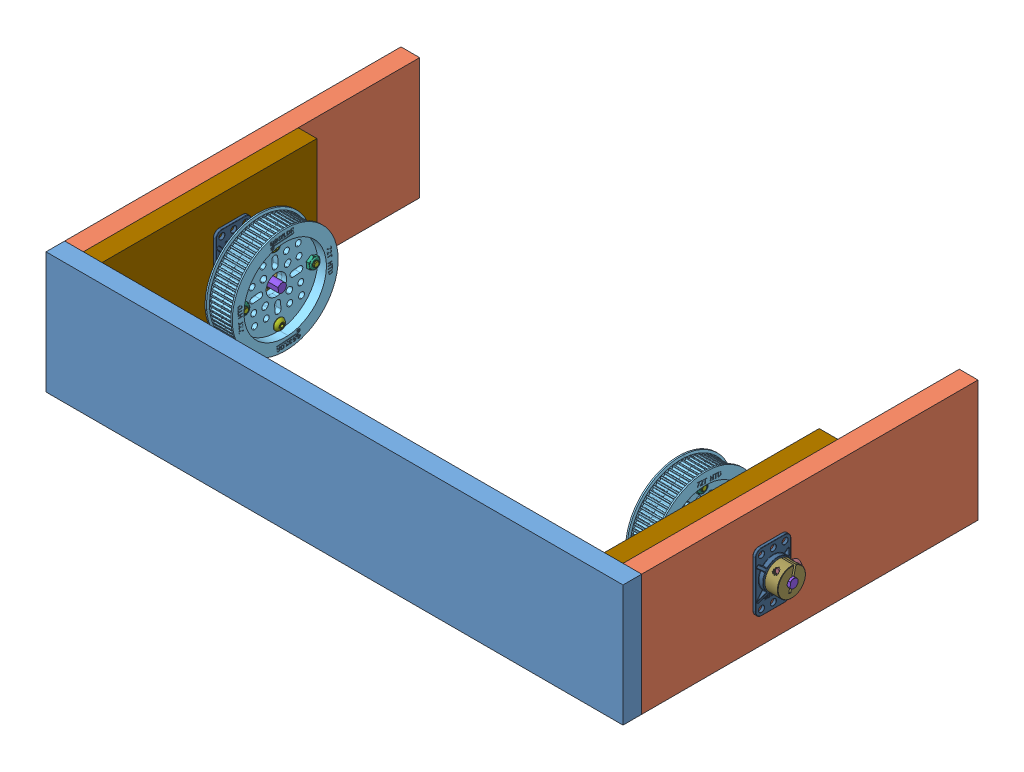
SolidWorks assembly hautElevateur, configuration Défaut. Lengths in mm.
Overall size (424.23 82.55 241.3).
75 component instances, 13 part files, 6 mates.
Components (placement in the parent):
- plaqueMoteurElevateur-1: plaqueMoteurElevateur [Défaut] at (-14.6749 -16.481 385.8661) size (392.22 82.55 12.7)
- pivotHautElevateur-1: pivotHautElevateur [Défaut] at (-183.2969 -207.8009 -55.2233) x (0 0 1) z (0 1 0) size (228.6 78.41 82.55)
  - plaqueHaut-1: plaqueHaut [Défaut] at (326.7894 -14.786 191.3199) x (1 0 0) z (0 -1 0) size (228.6 82.55 12.7)
  - 1309-0016-1006 assembly-1: 1309-0016-1006 assembly [Défaut] at (365.0893 27.1876 177.1992) x (0.655754 0 -0.754974) z (0 -1 0) size (28.36 32 10.95)
    - 1309-0016-1006 assembly.STEP-1: 1309-0016-1006 assembly.STEP [Défaut] at origin size (28.36 32 10.95)
      - 1309-0016-1006.STEP-1: 1309-0016-1006.STEP [Défaut] at (-18.2019 0.5776 8.7736) size (25.38 32 10)
      - 2800-0004-0014_90128A207.STEP-1: 2800-0004-0014_90128A207.STEP [Défaut] at (-16.149 11.6963 8.7736) x (0.5 -0.5 -0.707107) z (0.707107 0.707107 0) size (7 7 18.01)
      - 2800-0004-0014_90128A207.STEP-2: 2800-0004-0014_90128A207.STEP [Défaut] at (-20.2547 -10.5411 8.7736) x (-0.5 0.5 -0.707107) z (-0.707107 -0.707107 0) size (7 7 18.01)
  - 3402-0014-0072 pulley-1: 3402-0014-0072 pulley [Défaut] at (364.8802 56.6295 250.8953) x (0.070159 0 0.997536) z (0 -1 0) size (71.96 71.96 18.5)
    - 3402-0014-0072 assembly.STEP-1: 3402-0014-0072 assembly.STEP [Défaut] at origin size (71.96 71.96 18.5)
      - 3402-0014-0072.STEP-1: 3402-0014-0072.STEP [Défaut] at (-60.2208 7.0832 38.7155) size (71.96 71.96 10.5)
      - 3402-0014-0072.STEP-2: 3402-0014-0072.STEP [Défaut] at (-60.2208 7.0832 23.2155) x (0 -1 0) z (0 0 -1) size (71.96 71.96 10.5)
      - 2812-0004-0007_90576A103.STEP-1: 2812-0004-0007_90576A103.STEP [Défaut] at (-60.2208 31.0832 29.7155) x (0.866025 0.5 0) z (-0.5 0.866025 0) size (7.02 4.86 8.1)
      - 2812-0004-0007_90576A103.STEP-2: 2812-0004-0007_90576A103.STEP [Défaut] at (-60.2208 -16.9168 29.7155) x (0 1 0) z (-1 0 0) size (7.02 4.86 8.1)
      - 2812-0004-0007_90576A103.STEP-3: 2812-0004-0007_90576A103.STEP [Défaut] at (-84.2208 7.0832 32.2155) x (0.5 0.866025 0) z (0.866025 -0.5 0) size (7.02 4.86 8.1)
      - 2812-0004-0007_90576A103.STEP-4: 2812-0004-0007_90576A103.STEP [Défaut] at (-36.2208 7.0832 32.2155) x (1 0 0) z (0 -1 0) size (7.02 4.86 8.1)
      - 2802-0004-0010_92095A480.STEP-1: 2802-0004-0010_92095A480.STEP [Défaut] at (-36.2208 7.0832 25.5155) x (-0.923728 -0.383049 0) z (0 0 -1) size (13.53 12.99 15.57)
      - 2802-0004-0010_92095A480.STEP-2: 2802-0004-0010_92095A480.STEP [Défaut] at (-84.2208 7.0832 25.5155) x (0.923728 0.383049 0) z (0 0 -1) size (13.53 12.99 15.57)
      - 2802-0004-0010_92095A480.STEP-3: 2802-0004-0010_92095A480.STEP [Défaut] at (-60.2208 31.0832 36.4155) size (13.53 12.99 15.57)
      - 2802-0004-0010_92095A480.STEP-4: 2802-0004-0010_92095A480.STEP [Défaut] at (-60.2208 -16.9168 36.4155) x (-1 0 0) z (0 0 1) size (13.53 12.99 15.57)
  - 2101-0006-0300 3 po-1: 2101-0006-0300 3 po [Défaut] at (353.5894 -43.494 191.3199) x (0.070159 0 0.997536) z (-0.997536 0 0.070159) size (6 76.2 5.5)
  - blocHautCote-1: blocHautCote [Défaut] at (368.0644 -2.086 191.3199) x (1 0 0) z (0 -1 0) size (146.05 82.55 12.7)
  - 1616-0016-0002 plaque-1: 1616-0016-0002 plaque [Défaut] at (353.5894 -27.486 193.3199) size (24 5.02 40)
    - 1616-0016-0002.STEP-1: 1616-0016-0002.STEP [Défaut] at origin size (24 5.02 40)
      - 1616-0016-0002.STEP-1: 1616-0016-0002.STEP [Défaut] at origin size (24 5.02 40)
  - 1616-0016-0002 plaque-2: 1616-0016-0002 plaque [Défaut] at (353.5894 -2.086 193.3199) x (-1 0 0) z (0 0 1) size (24 5.02 40)
    - 1616-0016-0002.STEP-1: 1616-0016-0002.STEP [Défaut] at origin size (24 5.02 40)
      - 1616-0016-0002.STEP-1: 1616-0016-0002.STEP [Défaut] at origin size (24 5.02 40)
  - 1611-0514-0006 Roulement-1: 1611-0514-0006 Roulement [Défaut] at (353.5894 -32.486 191.3199) x (0.999897 0 0.014368) z (-0.014368 0 0.999897) size (15 5 15)
  - 2910-0919-0006 assembly collet-6: 2910-0919-0006 assembly collet [Défaut] at (379.8638 -36.9656 167.7839) x (0.972179 0 -0.234238) z (0.234238 0 0.972179) size (19 9.89 19.83)
    - 2910-0919-0006 assembly.STEP-1: 2910-0919-0006 assembly.STEP [Défaut] at origin size (19 9.89 19.83)
      - 2910-0919-0006.STEP-1: 2910-0919-0006.STEP [Défaut] at (-31.0565 -0.5204 16.7268) size (19 9.5 18.97)
      - 2800-0004-0010_90128A207.STEP-1: 2800-0004-0010_90128A207.STEP [Défaut] at (-24.2865 -0.5204 11.2868) x (0 -0.807243 -0.59022) z (1 0 0) size (7 7 14.01)
  - 1611-0514-0006 Roulement-2: 1611-0514-0006 Roulement [Défaut] at (353.5894 2.914 191.3199) x (-0.983829 0 -0.179109) z (-0.179109 0 0.983829) size (15 5 15)
  - 2910-0919-0006 assembly collet-7: 2910-0919-0006 assembly collet [Défaut] at (322.5329 7.3936 174.5931) x (-1 0 0) z (0 0 1) size (19 9.89 19.83)
    - 2910-0919-0006 assembly.STEP-1: 2910-0919-0006 assembly.STEP [Défaut] at origin size (19 9.89 19.83)
      - 2910-0919-0006.STEP-1: 2910-0919-0006.STEP [Défaut] at (-31.0565 -0.5204 16.7268) size (19 9.5 18.97)
      - 2800-0004-0010_90128A207.STEP-1: 2800-0004-0010_90128A207.STEP [Défaut] at (-24.2865 -0.5204 11.2868) x (0 -0.807243 -0.59022) z (1 0 0) size (7 7 14.01)
- pivotHautElevateur-2: pivotHautElevateur [Défaut] at (153.9472 174.8389 -55.2233) x (0 0 1) z (0 -1 0) size (228.6 78.41 82.55)
  - plaqueHaut-1: plaqueHaut [Défaut] at (326.7894 -14.786 191.3199) x (1 0 0) z (0 -1 0) size (228.6 82.55 12.7)
  - 1309-0016-1006 assembly-1: 1309-0016-1006 assembly [Défaut] at (365.0893 27.1876 177.1992) x (0.655754 0 -0.754974) z (0 -1 0) size (28.36 32 10.95)
    - 1309-0016-1006 assembly.STEP-1: 1309-0016-1006 assembly.STEP [Défaut] at origin size (28.36 32 10.95)
      - 1309-0016-1006.STEP-1: 1309-0016-1006.STEP [Défaut] at (-18.2019 0.5776 8.7736) size (25.38 32 10)
      - 2800-0004-0014_90128A207.STEP-1: 2800-0004-0014_90128A207.STEP [Défaut] at (-16.149 11.6963 8.7736) x (0.5 -0.5 -0.707107) z (0.707107 0.707107 0) size (7 7 18.01)
      - 2800-0004-0014_90128A207.STEP-2: 2800-0004-0014_90128A207.STEP [Défaut] at (-20.2547 -10.5411 8.7736) x (-0.5 0.5 -0.707107) z (-0.707107 -0.707107 0) size (7 7 18.01)
  - 3402-0014-0072 pulley-1: 3402-0014-0072 pulley [Défaut] at (364.8802 56.6295 250.8953) x (0.070159 0 0.997536) z (0 -1 0) size (71.96 71.96 18.5)
    - 3402-0014-0072 assembly.STEP-1: 3402-0014-0072 assembly.STEP [Défaut] at origin size (71.96 71.96 18.5)
      - 3402-0014-0072.STEP-1: 3402-0014-0072.STEP [Défaut] at (-60.2208 7.0832 38.7155) size (71.96 71.96 10.5)
      - 3402-0014-0072.STEP-2: 3402-0014-0072.STEP [Défaut] at (-60.2208 7.0832 23.2155) x (0 -1 0) z (0 0 -1) size (71.96 71.96 10.5)
      - 2812-0004-0007_90576A103.STEP-1: 2812-0004-0007_90576A103.STEP [Défaut] at (-60.2208 31.0832 29.7155) x (0.866025 0.5 0) z (-0.5 0.866025 0) size (7.02 4.86 8.1)
      - 2812-0004-0007_90576A103.STEP-2: 2812-0004-0007_90576A103.STEP [Défaut] at (-60.2208 -16.9168 29.7155) x (0 1 0) z (-1 0 0) size (7.02 4.86 8.1)
      - 2812-0004-0007_90576A103.STEP-3: 2812-0004-0007_90576A103.STEP [Défaut] at (-84.2208 7.0832 32.2155) x (0.5 0.866025 0) z (0.866025 -0.5 0) size (7.02 4.86 8.1)
      - 2812-0004-0007_90576A103.STEP-4: 2812-0004-0007_90576A103.STEP [Défaut] at (-36.2208 7.0832 32.2155) x (1 0 0) z (0 -1 0) size (7.02 4.86 8.1)
      - 2802-0004-0010_92095A480.STEP-1: 2802-0004-0010_92095A480.STEP [Défaut] at (-36.2208 7.0832 25.5155) x (-0.923728 -0.383049 0) z (0 0 -1) size (13.53 12.99 15.57)
      - 2802-0004-0010_92095A480.STEP-2: 2802-0004-0010_92095A480.STEP [Défaut] at (-84.2208 7.0832 25.5155) x (0.923728 0.383049 0) z (0 0 -1) size (13.53 12.99 15.57)
      - 2802-0004-0010_92095A480.STEP-3: 2802-0004-0010_92095A480.STEP [Défaut] at (-60.2208 31.0832 36.4155) size (13.53 12.99 15.57)
      - 2802-0004-0010_92095A480.STEP-4: 2802-0004-0010_92095A480.STEP [Défaut] at (-60.2208 -16.9168 36.4155) x (-1 0 0) z (0 0 1) size (13.53 12.99 15.57)
  - 2101-0006-0300 3 po-1: 2101-0006-0300 3 po [Défaut] at (353.5894 -43.494 191.3199) x (0.070159 0 0.997536) z (-0.997536 0 0.070159) size (6 76.2 5.5)
  - blocHautCote-1: blocHautCote [Défaut] at (368.0644 -2.086 191.3199) x (1 0 0) z (0 -1 0) size (146.05 82.55 12.7)
  - 1616-0016-0002 plaque-1: 1616-0016-0002 plaque [Défaut] at (353.5894 -27.486 193.3199) size (24 5.02 40)
    - 1616-0016-0002.STEP-1: 1616-0016-0002.STEP [Défaut] at origin size (24 5.02 40)
      - 1616-0016-0002.STEP-1: 1616-0016-0002.STEP [Défaut] at origin size (24 5.02 40)
  - 1616-0016-0002 plaque-2: 1616-0016-0002 plaque [Défaut] at (353.5894 -2.086 193.3199) x (-1 0 0) z (0 0 1) size (24 5.02 40)
    - 1616-0016-0002.STEP-1: 1616-0016-0002.STEP [Défaut] at origin size (24 5.02 40)
      - 1616-0016-0002.STEP-1: 1616-0016-0002.STEP [Défaut] at origin size (24 5.02 40)
  - 1611-0514-0006 Roulement-1: 1611-0514-0006 Roulement [Défaut] at (353.5894 -32.486 191.3199) x (0.999897 0 0.014368) z (-0.014368 0 0.999897) size (15 5 15)
  - 2910-0919-0006 assembly collet-6: 2910-0919-0006 assembly collet [Défaut] at (379.8638 -36.9656 167.7839) x (0.972179 0 -0.234238) z (0.234238 0 0.972179) size (19 9.89 19.83)
    - 2910-0919-0006 assembly.STEP-1: 2910-0919-0006 assembly.STEP [Défaut] at origin size (19 9.89 19.83)
      - 2910-0919-0006.STEP-1: 2910-0919-0006.STEP [Défaut] at (-31.0565 -0.5204 16.7268) size (19 9.5 18.97)
      - 2800-0004-0010_90128A207.STEP-1: 2800-0004-0010_90128A207.STEP [Défaut] at (-24.2865 -0.5204 11.2868) x (0 -0.807243 -0.59022) z (1 0 0) size (7 7 14.01)
  - 1611-0514-0006 Roulement-2: 1611-0514-0006 Roulement [Défaut] at (353.5894 2.914 191.3199) x (-0.983829 0 -0.179109) z (-0.179109 0 0.983829) size (15 5 15)
  - 2910-0919-0006 assembly collet-7: 2910-0919-0006 assembly collet [Défaut] at (322.5329 7.3936 174.5931) x (-1 0 0) z (0 0 1) size (19 9.89 19.83)
    - 2910-0919-0006 assembly.STEP-1: 2910-0919-0006 assembly.STEP [Défaut] at origin size (19 9.89 19.83)
      - 2910-0919-0006.STEP-1: 2910-0919-0006.STEP [Défaut] at (-31.0565 -0.5204 16.7268) size (19 9.5 18.97)
      - 2800-0004-0010_90128A207.STEP-1: 2800-0004-0010_90128A207.STEP [Défaut] at (-24.2865 -0.5204 11.2868) x (0 -0.807243 -0.59022) z (1 0 0) size (7 7 14.01)
Mates (geometry in assembly coordinates):
- Coïncidente23: coincident: plane of plaqueMoteurElevateur-1 through (-14.6749 -16.481 385.8661) normal (0 0 -1); plane of pivotHautElevateur-2/plaqueHaut-1 through (181.4332 -57.756 385.8661) normal (0 0 1)
- Coïncidente24: coincident: plane of plaqueMoteurElevateur-1 through (181.4332 24.794 398.5661) normal (1 0 0); plane of pivotHautElevateur-2/plaqueHaut-1 through (181.4332 -16.481 271.5661) normal (1 0 0)
- Coïncidente25: coincident: plane of plaqueMoteurElevateur-1 through (-210.7829 24.794 398.5661) normal (0 1 0); plane of pivotHautElevateur-2/plaqueHaut-1 through (181.4332 24.794 157.2661) normal (0 1 0)
- Coïncidente26: coincident: plane of plaqueMoteurElevateur-1 through (-14.6749 -16.481 385.8661) normal (0 0 -1); plane of pivotHautElevateur-1/plaqueHaut-1 through (-210.7829 24.794 385.8661) normal (0 0 1)
- Coïncidente27: coincident: plane of plaqueMoteurElevateur-1 through (-210.7829 24.794 398.5661) normal (0 1 0); plane of pivotHautElevateur-1/plaqueHaut-1 through (-210.7829 24.794 157.2661) normal (0 1 0)
- Coïncidente28: coincident: plane of plaqueMoteurElevateur-1 through (-210.7829 24.794 398.5661) normal (-1 0 0); plane of pivotHautElevateur-1/plaqueHaut-1 through (-210.7829 -16.481 271.5661) normal (-1 0 0)
